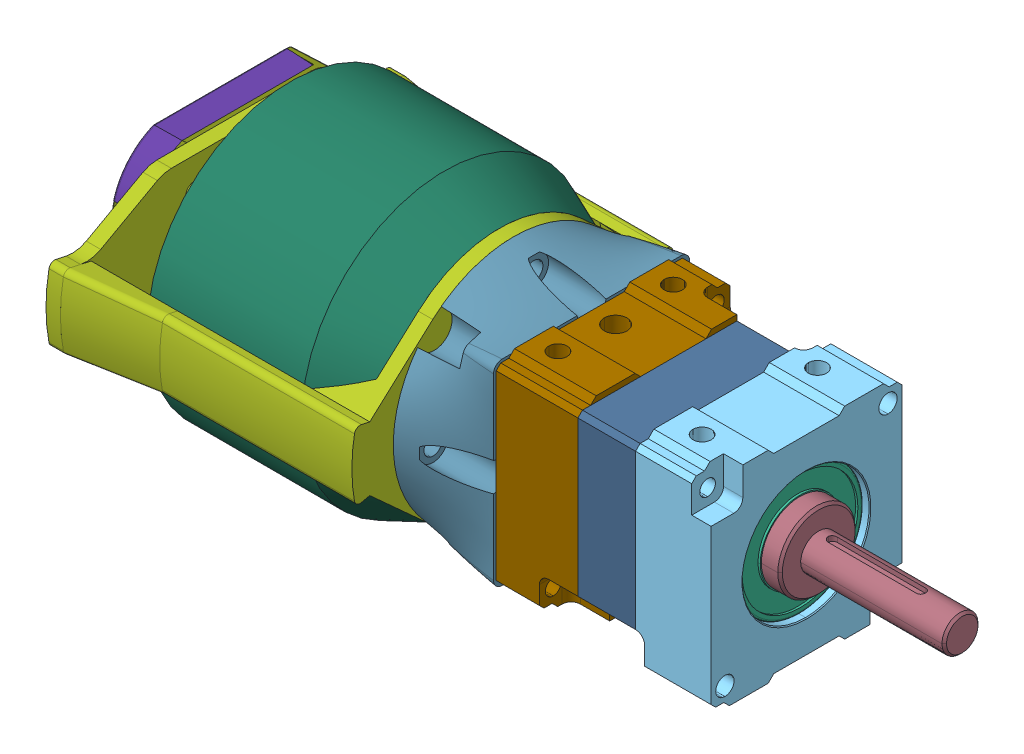
SolidWorks assembly Keda9to1, configuration Default. Lengths in mm.
Overall size (176.96 63 76.93).
46 component instances, 32 part files, 5 mates.
Components (placement in the parent):
- VersaPlanetary_v2_Single_Stage_10_1_with_BAG.STEP-1: VersaPlanetary_v2_Single_Stage_10_1_with_BAG.STEP [Default] at origin size (163.4 63.52 63.52)
  - 217-2820 Rev1_Public.STEP-1: 217-2820 Rev1_Public.STEP [Default] at (-4.6546 22.225 0) x (0 -0.456494 0.889726) z (-1 0 0) size (39.22 38.88 17.4)
    - 217-2625-100.STEP-1: 217-2625-100.STEP [Default] at origin size (39.22 38.88 12.7)
      - 217-2625-008 Rev1.STEP-1: 217-2625-008 Rev1.STEP [Default] at origin size (34.7 34.7 4.7)
      - 217-2625-010 Rev1.STEP-1: 217-2625-010 Rev1.STEP [Default] at (0 10.193 3.65) x (0.999813 0.019336 0) z (0 0 1) size (4 4 12)
      - 217-2625-010 Rev1.STEP-2: 217-2625-010 Rev1.STEP [Default] at (8.691 -5.3258 3.65) size (4 4 12)
      - 217-2625-010 Rev1.STEP-3: 217-2625-010 Rev1.STEP [Default] at (-8.691 -5.3258 3.65) size (4 4 12)
      - 217-2625-005 Rev1_Planet_Revolving_Follower01.STEP-1: 217-2625-005 Rev1_Planet_Revolving_Follower01.STEP [Default] at (8.691 -5.3258 6.35) x (0.932816 0.360354 0) z (0 0 1) size (16.89 16.89 8)
      - 217-2625-005 Rev1_Planet_Revolving_Follower01.STEP-2: 217-2625-005 Rev1_Planet_Revolving_Follower01.STEP [Default] at (-8.691 -5.3258 6.35) x (-0.932788 -0.360426 0) z (0 0 1) size (16.89 16.89 8)
      - 217-2625-005 Rev1_Planet_Revolving_Follower01.STEP-3: 217-2625-005 Rev1_Planet_Revolving_Follower01.STEP [Default] at (0 10.193 6.35) x (0.893583 0.448898 0) z (0 0 1) size (16.89 16.89 8)
    - 217-2625-007 Rev1_Public.STEP-1: 217-2625-007 Rev1_Public.STEP [Default] at (0 0 6.7) x (0.992772 0.120019 0) z (0 0 1) size (15.27 15.27 12.7)
  - 217-2625-026 Rev1.STEP-1: 217-2625-026 Rev1.STEP [Default] at (-6.5 22.225 0) x (0 -1 0) z (-1 0 0) size (44.45 42 18.12)
  - 217-2742-001 Rev4.STEP-1: 217-2742-001 Rev4.STEP [Default] at (0.2002 22.225 0) x (1 0 0) z (0 -0.092627 0.995701) size (7 28 28)
  - 217-2742-001 Rev4.STEP-2: 217-2742-001 Rev4.STEP [Default] at (8.2002 22.225 0) size (7 28 28)
  - 217-2625-017 Rev1_9714K61.STEP-1: 217-2625-017 Rev1_9714K61.STEP [Default] at (7.42 22.3002 -0.342) x (0 0.56703 0.823697) z (0 -0.823697 0.56703) size (28.51 4.98 27.43)
  - 217-2625-003 Rev1.STEP-1: 217-2625-003 Rev1.STEP [Default] at (7.4478 22.225 0) x (0 -1 0) z (1 0 0) size (17 17 64.11) (hidden)
  - 217-2625-018 Rev1_98541A410.STEP-1: 217-2625-018 Rev1_98541A410.STEP [Default] at (-0.7046 22.225 0) x (1 0 0) z (0 -0.017452 0.999848) size (1 19.6 17.4)
  - 832-1750-Ring-Gear-Screw_SSA0832-0500ZC.STEP-1: 832-1750-Ring-Gear-Screw_SSA0832-0500ZC.STEP [Default] at (-30.7 4.725 -17.5) x (0 0.997447 0.071411) z (0 -0.071411 0.997447) size (6.73 48.51 6.73) (hidden)
  - 832-1750-Ring-Gear-Screw_SSA0832-0500ZC.STEP-2: 832-1750-Ring-Gear-Screw_SSA0832-0500ZC.STEP [Default] at (-30.7 39.725 17.5) x (0 0.005929 0.999982) z (0 -0.999982 0.005929) size (6.73 48.51 6.73) (hidden)
  - 217-2625-025 Rev1.STEP-1: 217-2625-025 Rev1.STEP [Default] at (-23.2 22.225 0) x (0 -1 0) z (-1 0 0) size (44.45 42 18)
  - 217-4649-002 Rev1_SSA0832-0500ZC.STEP-1: 217-4649-002 Rev1_SSA0832-0500ZC.STEP [Default] at (-33.7 4.2645 17.9605) x (0 0.33842 -0.940995) z (0 0.940995 0.33842) size (6.73 16.76 6.73) (hidden)
  - 217-4649-002 Rev1_SSA0832-0500ZC.STEP-2: 217-4649-002 Rev1_SSA0832-0500ZC.STEP [Default] at (-33.7 40.1855 -17.9605) x (0 -0.308932 -0.951084) z (0 0.951084 -0.308932) size (6.73 16.76 6.73) (hidden)
  - 217-4649-006 Rev1_SSA0004-008BA.STEP-1: 217-4649-006 Rev1_SSA0004-008BA.STEP [Default] at (-30.7 22.225 12.5) x (0 0.5 -0.866025) z (0 -0.866025 -0.5) size (7 14 7) (hidden)
  - 217-4649-006 Rev1_SSA0004-008BA.STEP-2: 217-4649-006 Rev1_SSA0004-008BA.STEP [Default] at (-30.7 22.225 -12.5) x (0 -0.5 0.866025) z (0 0.866025 0.5) size (7 14 7) (hidden)
  - 217-2822-003 Rev4.STEP-1: 217-2822-003 Rev4.STEP [Default] at (-32.2 22.225 0) x (0 -1 0) z (-1 0 0) size (42 42 4.8) (hidden)
  - 217-3351 Rev2.STEP-1: 217-3351 Rev2.STEP [Default] at (-33.7 22.225 0) x (0 0 1) z (1 0 0) size (59.07 59.07 84.5) (hidden)
  - 217-2816-001 Rev1.STEP-1: 217-2816-001 Rev1.STEP [Default] at (-6.35 22.225 0) x (0 -1 0) z (1 0 0) size (42 42 14.51)
  - 217-4649-001 Rev1.STEP-1: 217-4649-001 Rev1.STEP [Default] at (-20.046 22.225 0) x (0 -1 0) z (1 0 0) size (18 18 13)
  - 217-4649-007 Rev1_94105A824.STEP-1: 217-4649-007 Rev1_94105A824.STEP [Default] at (-25.521 22.225 -6.7835) x (-0.996104 -0.088191 0) z (0 0 -1) size (4.83 4.83 4.77)
  - 217-2625-011 Rev1.STEP-1: 217-2625-011 Rev1.STEP [Default] at (-24.7818 22.225 0) x (0 0 1) z (0 -1 0) size (8.01 7.5 7.94) (hidden)
- VersaPlanetary_CIM_Motor_Output_Shaft_Kit_217-2893-1: VersaPlanetary_CIM_Motor_Output_Shaft_Kit_217-2893 [Default] at (7.4478 22.225 0) x (0 0 -1) z (1 0 0) size (17 17 57.85)
- KedaAdapter^Keda9to1-1: KedaAdapter^Keda9to1 [Default] at origin size (17.82 53.01 53.01) (virtual)
- 192kvMotorEncoded-1: 192kvMotorEncoded [Default] at (-51.0318 22.225 0) x (0 -1 0) z (0 0 -1) size (63 104.52 76.93)
  - BetterKEDA-1: BetterKEDA [Default] at origin size (63 104.52 63)
  - CUI_DEVICES_AMT102-0048-N2000-S-1: CUI_DEVICES_AMT102-0048-N2000-S [Default] at (0 65.12 0) x (1 0 0) z (0 1 0) size (36.33 46.21 9.2)
    - CUI_DEVICES_AMT102-0048-N2000-S.step-1: CUI_DEVICES_AMT102-0048-N2000-S.step [Default] at origin size (36.33 46.21 9.2)
      - AMT-102-Base-REV-K.step-1: AMT-102-Base-REV-K.step [Default] x (-1 0 0) z (0 0 -1) size (28.78 43.39 9.06)
      - AMT-102-Top-Cover-REV-H.step-1: AMT-102-Top-Cover-REV-H.step [Default] at (0 0 5.23) x (-1 0 0) z (0 0 -1) size (28.6 43.26 6.55)
      - AMT-Sleeve-REV-D_ 2 mm.step-1: AMT-Sleeve-REV-D_ 2 mm.step [Default] at (0 0 -2.42) x (0.999996 0.002864 0) z (0 0 1) size (10.79 10.79 7.8)
      - AMT-Hub-Top-REV-D1.step-1: AMT-Hub-Top-REV-D1.step [Default] at (0 0 2.13) x (0.999996 0.002864 0) z (0 0 1) size (14 14 5.67)
      - AMT-Hub-Bottom-REV-B.step-1: AMT-Hub-Bottom-REV-B.step [Default] at (0 0 2.43) x (0.999998 -0.001942 0) z (0 0 1) size (17.3 17.3 3.2)
      - AMT10X-Shaft-Adaptor-REV-E.step-1: AMT10X-Shaft-Adaptor-REV-E.step [Default] at (0 0 0.03) x (0.999996 0.002864 0) z (0 0 1) size (11.8 11.8 7.8)
      - Receiver-board.step-1: Receiver-board.step [Default] at (72.2834 -20.351 3.03) x (-1 0 0) z (0 0 -1) size (26.5 26.62 0.41)
      - Rotor-board-REV F.step-1: Rotor-board-REV F.step [Default] at (0 0 2.13) x (0.807874 -0.589355 0) z (0 0 1) size (26 26 0.3)
      - Transmitter-board AMT10_AMT-102.step-1: Transmitter-board AMT10_AMT-102.step [Default] at (19.1596 -17.1102 1.22) x (-1 0 0) z (0 0 -1) size (26.63 38.43 4.41)
  - Body^192kvMotorEncoded-1: Body^192kvMotorEncoded [Default] at origin size (53 64.53 76.93) (virtual)
Mates (geometry in assembly coordinates):
- Concentric2: concentric anti-aligned: cylinder of VersaPlanetary_v2_Single_Stage_10_1_with_BAG.STEP-1/217-2742-001 Rev4.STEP-2 through (8.2002 22.225 0) axis (-1 0 0) radius 7.5; cylinder of VersaPlanetary_CIM_Motor_Output_Shaft_Kit_217-2893-1 through (15.2002 22.225 0) axis (1 0 0) radius 8.5
- Coincident3: coincident anti-aligned: plane of VersaPlanetary_v2_Single_Stage_10_1_with_BAG.STEP-1/217-2742-001 Rev4.STEP-2 through (15.2002 29.725 0) normal (1 0 0); plane of VersaPlanetary_CIM_Motor_Output_Shaft_Kit_217-2893-1 through (15.2002 22.225 0) normal (-1 0 0)
- Concentric3: concentric aligned: cylinder of VersaPlanetary_v2_Single_Stage_10_1_with_BAG.STEP-1/217-4649-001 Rev1.STEP-1 through (-20.046 22.225 0) axis (-1 0 0) radius 4.005; cylinder of MotorEncoded-1/BetterKEDA-1 through (-21.5068 22.225 0) axis (-1 0 0) radius 4
- Coincident4: coincident anti-aligned: plane of KedaAdapter^VersaPlanetary_v2_Single_Stage_9_1_with_BAG-1 through (-51.0318 0 0) normal (-1 0 0); plane of MotorEncoded-1/BetterKEDA-1 through (-51.0318 22.225 0) normal (1 0 0)
- Coincident5: coincident anti-aligned: plane of 192kvMotorEncoded-1 through (-51.0318 22.225 0) normal (0 0 -1)
